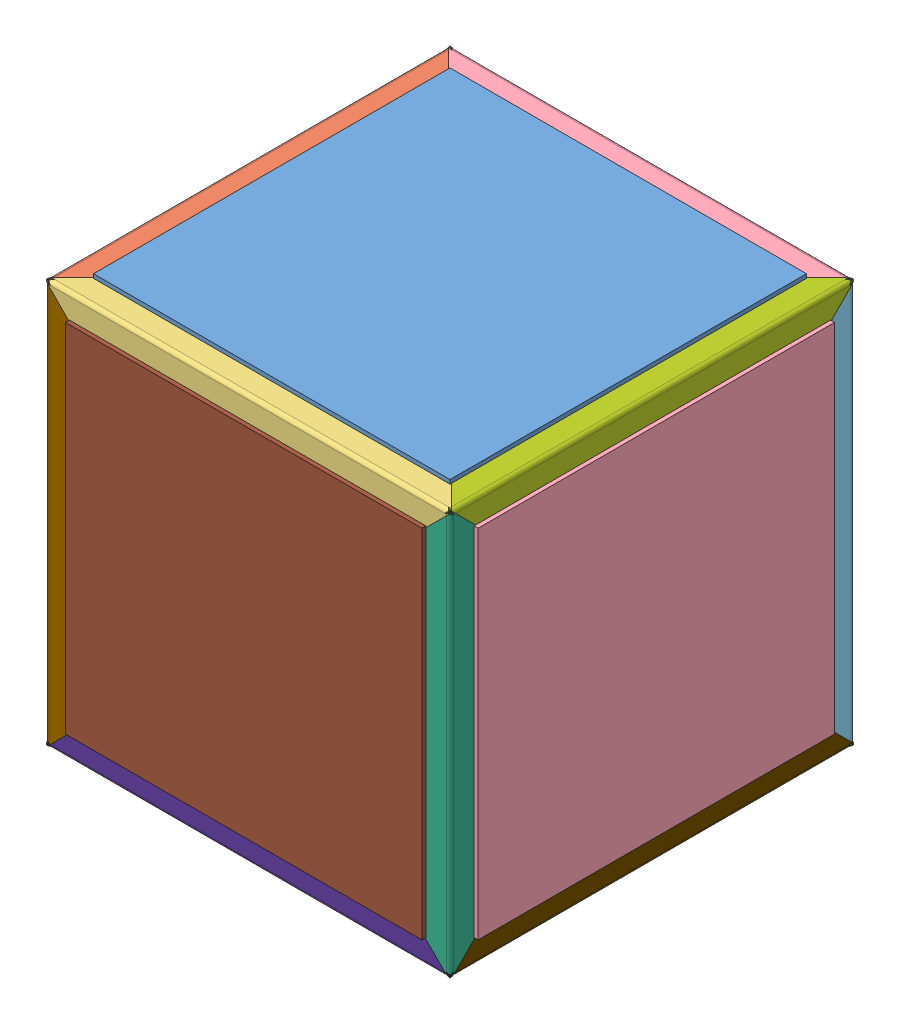
SolidWorks assembly cube_01, configuration cube01. Lengths in mm.
Overall size (163.19 163.19 163.19).
30 component instances, 30 part files, 92 mates.
Components (placement in the parent):
- pr^cube_01-28: pr^cube_01 [cube01] x (-1 0 0) z (0 0 1) size (140.97 1.59 140.97) (virtual)
- dr1^cube_01-55: dr1^cube_01 [cube01] at (-79.4046 80.01 0) x (0 -1 0) z (0 0 1) size (26.01 26.01 160.03) (virtual)
- dr2^cube_01-37: dr2^cube_01 [cube01] at (0 80.01 79.4046) x (0 -1 0) z (1 0 0) size (26.01 26.01 160.03) (virtual)
- dr3^cube_01-33: dr3^cube_01 [cube01] at (0 80.01 -79.4046) x (0 -1 0) z (-1 0 0) size (26.01 26.01 160.03) (virtual)
- br1^cube_01-49: br1^cube_01 [Default] at (0 54.61 -54.61) x (0 0 1) z (-1 0 0) size (50.8 50.8 102.11) (virtual)
- br2^cube_01-61: br2^cube_01 [Default] at (-54.61 54.61 0) size (50.8 50.8 102.11) (virtual)
- br3^cube_01-46: br3^cube_01 [Default] at (0 54.61 54.61) x (0 0 -1) z (1 0 0) size (50.8 50.8 102.11) (virtual)
- pg^cube_01-20: pg^cube_01 [cube01] x (0 -1 0) z (0 0 1) size (140.97 1.59 140.97) (virtual)
- dg1^cube_01-38: dg1^cube_01 [cube01] at (-80.01 0 79.4046) x (1 0 0) z (0 1 0) size (26.01 26.01 160.03) (virtual)
- dg2^cube_01-41: dg2^cube_01 [cube01] at (-80.01 -79.4046 0) size (26.01 26.01 160.03) (virtual)
- dg3^cube_01-34: dg3^cube_01 [cube01] at (-80.01 0 -79.4046) x (1 0 0) z (0 -1 0) size (26.01 26.01 160.03) (virtual)
- bg1^cube_01-47: bg1^cube_01 [Default] at (-54.61 -54.61 0) x (0 1 0) z (0 0 1) size (50.8 50.8 102.11) (virtual)
- bg2^cube_01-44: bg2^cube_01 [Default] at (-54.61 0 54.61) x (0 0 -1) z (0 1 0) size (50.8 50.8 102.11) (virtual)
- bg3^cube_01-40: bg3^cube_01 [Default] at (-54.61 0 -54.61) x (0 0 1) z (0 -1 0) size (50.8 50.8 102.11) (virtual)
- py^cube_01-21: py^cube_01 [cube01] at origin size (140.97 1.59 140.97) (virtual)
- dy1^cube_01-35: dy1^cube_01 [cube01] at (0 -80.01 -79.4046) x (0 1 0) z (1 0 0) size (26.01 26.01 160.03) (virtual)
- dy2^cube_01-39: dy2^cube_01 [cube01] at (0 -80.01 79.4046) x (0 1 0) z (-1 0 0) size (26.01 26.01 160.03) (virtual)
- dy3^cube_01-42: dy3^cube_01 [cube01] at (79.4046 -80.01 0) x (0 1 0) z (0 0 1) size (26.01 26.01 160.03) (virtual)
- by1^cube_01-41: by1^cube_01 [Default] at (0 -54.61 -54.61) x (0 0 1) z (1 0 0) size (50.8 50.8 102.11) (virtual)
- by2^cube_01-45: by2^cube_01 [Default] at (0 -54.61 54.61) x (0 0 -1) z (-1 0 0) size (50.8 50.8 102.11) (virtual)
- by3^cube_01-48: by3^cube_01 [Default] at (54.61 -54.61 0) x (-1 0 0) z (0 0 1) size (50.8 50.8 102.11) (virtual)
- po^cube_01-22: po^cube_01 [cube01] x (0 1 0) z (0 0 1) size (140.97 1.59 140.97) (virtual)
- do1^cube_01-36: do1^cube_01 [cube01] at (80.01 0 -79.4046) x (-1 0 0) z (0 1 0) size (26.01 26.01 160.03) (virtual)
- do2^cube_01-40: do2^cube_01 [cube01] at (80.01 0 79.4046) x (-1 0 0) z (0 -1 0) size (26.01 26.01 160.03) (virtual)
- do3^cube_01-47: do3^cube_01 [cube01] at (80.01 79.4046 0) x (-1 0 0) z (0 0 1) size (26.01 26.01 160.03) (virtual)
- bo1^cube_01-42: bo1^cube_01 [Default] at (54.61 0 -54.61) x (0 0 1) z (0 1 0) size (50.8 50.8 102.11) (virtual)
- bo2^cube_01-46: bo2^cube_01 [Default] at (54.61 0 54.61) x (0 0 -1) z (0 -1 0) size (50.8 50.8 102.11) (virtual)
- bo3^cube_01-62: bo3^cube_01 [Default] at (54.61 54.61 0) x (0 -1 0) z (0 0 1) size (50.8 50.8 102.11) (virtual)
- pc^cube_01-18: pc^cube_01 [cube01] x (-1 0 0) z (0 -1 0) size (140.97 1.59 140.97) (virtual)
- pb^cube_01-21: pb^cube_01 [cube01] x (-1 0 0) z (0 1 0) size (140.97 1.59 140.97) (virtual)
Mates (geometry in assembly coordinates):
- Coincident1: coincident anti-aligned: plane of pr^cube_01-28 through (70.485 80.01 -70.485) normal (0 -1 0); plane of br1^cube_01-49 through (-51.054 80.01 -54.61) normal (0 1 0)
- Coincident2: coincident anti-aligned: plane of pr^cube_01-28 through (70.485 80.01 -70.485) normal (0 -1 0); plane of br2^cube_01-61 through (-54.61 80.01 51.054) normal (0 1 0)
- Coincident3: coincident anti-aligned: plane of pr^cube_01-28 through (70.485 80.01 -70.485) normal (0 -1 0); plane of br3^cube_01-46 through (51.054 80.01 54.61) normal (0 1 0)
- Coincident4: coincident anti-aligned: plane of pr^cube_01-28 through (70.485 80.01 -70.485) normal (0 -1 0); plane of bo3^cube_01-62 through (54.61 80.01 51.054) normal (0 1 0)
- Coincident5: coincident anti-aligned: plane of pr^cube_01-28 through (70.485 80.01 -70.485) normal (0 -1 0); plane of dr3^cube_01-33 through (0 80.01 -159.4146) normal (0 1 0)
- Coincident6: coincident anti-aligned: plane of pr^cube_01-28 through (70.485 80.01 -70.485) normal (0 -1 0); plane of dr1^cube_01-55 through (-159.4146 80.01 0) normal (0 1 0)
- Coincident7: coincident anti-aligned: plane of pr^cube_01-28 through (70.485 80.01 -70.485) normal (0 -1 0); plane of do3^cube_01-47 through (-0.6054 80.01 0) normal (0 1 0)
- Coincident8: coincident anti-aligned: plane of pr^cube_01-28 through (70.485 80.01 -70.485) normal (0 -1 0); plane of dr2^cube_01-37 through (0 80.01 159.4146) normal (0 1 0)
- Coincident34: coincident anti-aligned: plane of pb^cube_01-21 through (70.485 -70.485 -80.01) normal (0 0 1); plane of by1^cube_01-41 through (51.054 -54.61 -80.01) normal (0 0 -1)
- Coincident35: coincident anti-aligned: plane of pb^cube_01-21 through (70.485 -70.485 -80.01) normal (0 0 1); plane of bo1^cube_01-42 through (54.61 51.054 -80.01) normal (0 0 -1)
- Coincident36: coincident anti-aligned: plane of pb^cube_01-21 through (70.485 -70.485 -80.01) normal (0 0 1); plane of br1^cube_01-49 through (-51.054 54.61 -80.01) normal (0 0 -1)
- Coincident37: coincident anti-aligned: plane of pb^cube_01-21 through (70.485 -70.485 -80.01) normal (0 0 1); plane of bg3^cube_01-40 through (-54.61 -51.054 -80.01) normal (0 0 -1)
- Coincident38: coincident anti-aligned: plane of pb^cube_01-21 through (70.485 -70.485 -80.01) normal (0 0 1); plane of dg3^cube_01-34 through (0.6054 0 -80.01) normal (0 0 -1)
- Coincident39: coincident anti-aligned: plane of pb^cube_01-21 through (70.485 -70.485 -80.01) normal (0 0 1); plane of dr3^cube_01-33 through (0 -0.6054 -80.01) normal (0 0 -1)
- Coincident40: coincident anti-aligned: plane of pb^cube_01-21 through (70.485 -70.485 -80.01) normal (0 0 1); plane of do1^cube_01-36 through (-0.6054 0 -80.01) normal (0 0 -1)
- Coincident41: coincident anti-aligned: plane of pb^cube_01-21 through (70.485 -70.485 -80.01) normal (0 0 1); plane of dy1^cube_01-35 through (0 0.6054 -80.01) normal (0 0 -1)
- Coincident42: coincident anti-aligned: plane of pc^cube_01-18 through (70.485 70.485 80.01) normal (0 0 -1); plane of bo2^cube_01-46 through (54.61 -51.054 80.01) normal (0 0 1)
- Coincident43: coincident anti-aligned: plane of pc^cube_01-18 through (70.485 70.485 80.01) normal (0 0 -1); plane of br3^cube_01-46 through (51.054 54.61 80.01) normal (0 0 1)
- Coincident44: coincident anti-aligned: plane of pc^cube_01-18 through (70.485 70.485 80.01) normal (0 0 -1); plane of bg2^cube_01-44 through (-54.61 51.054 80.01) normal (0 0 1)
- Coincident45: coincident anti-aligned: plane of pc^cube_01-18 through (70.485 70.485 80.01) normal (0 0 -1); plane of by2^cube_01-45 through (-51.054 -54.61 80.01) normal (0 0 1)
- Coincident46: coincident anti-aligned: plane of pc^cube_01-18 through (70.485 70.485 80.01) normal (0 0 -1); plane of do2^cube_01-40 through (-0.6054 0 80.01) normal (0 0 1)
- Coincident47: coincident anti-aligned: plane of pc^cube_01-18 through (70.485 70.485 80.01) normal (0 0 -1); plane of dy2^cube_01-39 through (0 0.6054 80.01) normal (0 0 1)
- Coincident48: coincident anti-aligned: plane of pc^cube_01-18 through (70.485 70.485 80.01) normal (0 0 -1); plane of dg1^cube_01-38 through (0.6054 0 80.01) normal (0 0 1)
- Coincident49: coincident anti-aligned: plane of pc^cube_01-18 through (70.485 70.485 80.01) normal (0 0 -1); plane of dr2^cube_01-37 through (0 -0.6054 80.01) normal (0 0 1)
- Coincident50: coincident anti-aligned: plane of pg^cube_01-20 through (-80.01 70.485 -70.485) normal (1 0 0); plane of bg3^cube_01-40 through (-80.01 -51.054 -54.61) normal (-1 0 0)
- Coincident51: coincident anti-aligned: plane of pg^cube_01-20 through (-80.01 70.485 -70.485) normal (1 0 0); plane of bg1^cube_01-47 through (-80.01 -54.61 51.054) normal (-1 0 0)
- Coincident52: coincident anti-aligned: plane of pg^cube_01-20 through (-80.01 70.485 -70.485) normal (1 0 0); plane of bg2^cube_01-44 through (-80.01 51.054 54.61) normal (-1 0 0)
- Coincident53: coincident anti-aligned: plane of pg^cube_01-20 through (-80.01 70.485 -70.485) normal (1 0 0); plane of dr1^cube_01-55 through (-80.01 -0.6054 0) normal (-1 0 0)
- Coincident54: coincident anti-aligned: plane of pg^cube_01-20 through (-80.01 70.485 -70.485) normal (1 0 0); plane of dg3^cube_01-34 through (-80.01 0 -159.4146) normal (-1 0 0)
- Coincident55: coincident anti-aligned: plane of pg^cube_01-20 through (-80.01 70.485 -70.485) normal (1 0 0); plane of dg2^cube_01-41 through (-80.01 -159.4146 0) normal (-1 0 0)
- Coincident56: coincident anti-aligned: plane of pg^cube_01-20 through (-80.01 70.485 -70.485) normal (1 0 0); plane of dg1^cube_01-38 through (-80.01 0 159.4146) normal (-1 0 0)
- Coincident99: coincident anti-aligned: plane of pg^cube_01-20 through (-80.01 70.485 -70.485) normal (1 0 0); plane of br2^cube_01-61 through (-80.01 54.61 51.054) normal (-1 0 0)
- Coincident57: coincident anti-aligned: plane of py^cube_01-21 through (-70.485 -80.01 -70.485) normal (0 1 0); plane of by3^cube_01-48 through (54.61 -80.01 51.054) normal (0 -1 0)
- Coincident58: coincident anti-aligned: plane of py^cube_01-21 through (-70.485 -80.01 -70.485) normal (0 1 0); plane of by2^cube_01-45 through (-51.054 -80.01 54.61) normal (0 -1 0)
- Coincident59: coincident anti-aligned: plane of py^cube_01-21 through (-70.485 -80.01 -70.485) normal (0 1 0); plane of bg1^cube_01-47 through (-54.61 -80.01 51.054) normal (0 -1 0)
- Coincident60: coincident anti-aligned: plane of py^cube_01-21 through (-70.485 -80.01 -70.485) normal (0 1 0); plane of by1^cube_01-41 through (51.054 -80.01 -54.61) normal (0 -1 0)
- Coincident61: coincident anti-aligned: plane of py^cube_01-21 through (-70.485 -80.01 -70.485) normal (0 1 0); plane of dy3^cube_01-42 through (159.4146 -80.01 0) normal (0 -1 0)
- Coincident62: coincident anti-aligned: plane of py^cube_01-21 through (-70.485 -80.01 -70.485) normal (0 1 0); plane of dy2^cube_01-39 through (0 -80.01 159.4146) normal (0 -1 0)
- Coincident63: coincident anti-aligned: plane of py^cube_01-21 through (-70.485 -80.01 -70.485) normal (0 1 0); plane of dg2^cube_01-41 through (0.6054 -80.01 0) normal (0 -1 0)
- Coincident64: coincident anti-aligned: plane of py^cube_01-21 through (-70.485 -80.01 -70.485) normal (0 1 0); plane of dy1^cube_01-35 through (0 -80.01 -159.4146) normal (0 -1 0)
- Coincident65: coincident anti-aligned: plane of po^cube_01-22 through (80.01 -70.485 -70.485) normal (-1 0 0); plane of bo1^cube_01-42 through (80.01 51.054 -54.61) normal (1 0 0)
- Coincident66: coincident anti-aligned: plane of po^cube_01-22 through (80.01 -70.485 -70.485) normal (-1 0 0); plane of by3^cube_01-48 through (80.01 -54.61 51.054) normal (1 0 0)
- Coincident67: coincident anti-aligned: plane of po^cube_01-22 through (80.01 -70.485 -70.485) normal (-1 0 0); plane of bo2^cube_01-46 through (80.01 -51.054 54.61) normal (1 0 0)
- Coincident68: coincident anti-aligned: plane of po^cube_01-22 through (80.01 -70.485 -70.485) normal (-1 0 0); plane of bo3^cube_01-62 through (80.01 54.61 51.054) normal (1 0 0)
- Coincident69: coincident anti-aligned: plane of po^cube_01-22 through (80.01 -70.485 -70.485) normal (-1 0 0); plane of do2^cube_01-40 through (80.01 0 159.4146) normal (1 0 0)
- Coincident70: coincident anti-aligned: plane of po^cube_01-22 through (80.01 -70.485 -70.485) normal (-1 0 0); plane of do3^cube_01-47 through (80.01 159.4146 0) normal (1 0 0)
- Coincident71: coincident anti-aligned: plane of po^cube_01-22 through (80.01 -70.485 -70.485) normal (-1 0 0); plane of do1^cube_01-36 through (80.01 0 -159.4146) normal (1 0 0)
- Coincident72: coincident anti-aligned: plane of po^cube_01-22 through (80.01 -70.485 -70.485) normal (-1 0 0); plane of dy3^cube_01-42 through (80.01 0.6054 0) normal (1 0 0)
- Coincident73: coincident aligned: plane of assembly through (0 0 0) normal (0 0 1); plane of dy3^cube_01-42 through (79.4046 -80.01 0) normal (0 0 1)
- Coincident74: coincident aligned: plane of assembly through (0 0 0) normal (0 0 1); plane of by3^cube_01-48 through (54.61 -54.61 0) normal (0 0 1)
- Coincident75: coincident aligned: plane of assembly through (0 0 0) normal (0 0 1); plane of bo3^cube_01-62 through (54.61 54.61 0) normal (0 0 1)
- Coincident76: coincident aligned: plane of assembly through (0 0 0) normal (0 0 1); plane of do3^cube_01-47 through (80.01 79.4046 0) normal (0 0 1)
- Coincident77: coincident aligned: plane of assembly through (0 0 0) normal (0 0 1); plane of dg2^cube_01-41 through (-80.01 -79.4046 0) normal (0 0 1)
- Coincident78: coincident aligned: plane of assembly through (0 0 0) normal (0 0 1); plane of bg1^cube_01-47 through (-54.61 -54.61 0) normal (0 0 1)
- Coincident79: coincident aligned: plane of assembly through (0 0 0) normal (0 0 1); plane of dr1^cube_01-55 through (-79.4046 80.01 0) normal (0 0 1)
- Coincident80: coincident aligned: plane of assembly through (0 0 0) normal (0 0 1); plane of br2^cube_01-61 through (-54.61 54.61 0) normal (0 0 1)
- Coincident81: coincident aligned: plane of assembly through (0 0 0) normal (0 1 0); plane of bo1^cube_01-42 through (54.61 0 -54.61) normal (0 1 0)
- Coincident82: coincident aligned: plane of assembly through (0 0 0) normal (0 1 0); plane of py^cube_01-21 through (0 0 0) normal (0 1 0)
- Coincident83: coincident aligned: plane of assembly through (0 0 0) normal (0 1 0); plane of do1^cube_01-36 through (80.01 0 -79.4046) normal (0 1 0)
- Coincident84: coincident anti-aligned: plane of assembly through (0 0 0) normal (0 1 0); plane of bg3^cube_01-40 through (-54.61 0 -54.61) normal (0 -1 0)
- Coincident85: coincident anti-aligned: plane of assembly through (0 0 0) normal (0 1 0); plane of dg3^cube_01-34 through (-80.01 0 -79.4046) normal (0 -1 0)
- Coincident86: coincident aligned: plane of assembly through (0 0 0) normal (0 1 0); plane of dg1^cube_01-38 through (-80.01 0 79.4046) normal (0 1 0)
- Coincident87: coincident aligned: plane of assembly through (0 0 0) normal (0 1 0); plane of bg2^cube_01-44 through (-54.61 0 54.61) normal (0 1 0)
- Coincident88: coincident anti-aligned: plane of assembly through (0 0 0) normal (0 1 0); plane of bo2^cube_01-46 through (54.61 0 54.61) normal (0 -1 0)
- Coincident89: coincident anti-aligned: plane of assembly through (0 0 0) normal (0 1 0); plane of do2^cube_01-40 through (80.01 0 79.4046) normal (0 -1 0)
- Coincident90: coincident anti-aligned: plane of assembly through (0 0 0) normal (1 0 0); plane of by2^cube_01-45 through (0 -54.61 54.61) normal (-1 0 0)
- Coincident91: coincident anti-aligned: plane of assembly through (0 0 0) normal (1 0 0); plane of dy2^cube_01-39 through (0 -80.01 79.4046) normal (-1 0 0)
- Coincident92: coincident aligned: plane of assembly through (0 0 0) normal (1 0 0); plane of pg^cube_01-20
- Coincident93: coincident aligned: plane of assembly through (0 0 0) normal (1 0 0); plane of dr2^cube_01-37 through (0 80.01 79.4046) normal (1 0 0)
- Coincident94: coincident aligned: plane of assembly through (0 0 0) normal (1 0 0); plane of br3^cube_01-46 through (0 54.61 54.61) normal (1 0 0)
- Coincident95: coincident anti-aligned: plane of assembly through (0 0 0) normal (1 0 0); plane of dr3^cube_01-33 through (0 80.01 -79.4046) normal (-1 0 0)
- Coincident96: coincident anti-aligned: plane of assembly through (0 0 0) normal (1 0 0); plane of br1^cube_01-49 through (0 54.61 -54.61) normal (-1 0 0)
- Coincident97: coincident aligned: plane of assembly through (0 0 0) normal (1 0 0); plane of by1^cube_01-41 through (0 -54.61 -54.61) normal (1 0 0)
- Coincident98: coincident aligned: plane of assembly through (0 0 0) normal (1 0 0); plane of dy1^cube_01-35 through (0 -80.01 -79.4046) normal (1 0 0)
- Coincident100: coincident anti-aligned: plane of pr^cube_01-28; plane of assembly through (0 0 0) normal (1 0 0)
- Coincident101: coincident aligned: plane of pr^cube_01-28 through (0 0 0) normal (0 0 1); plane of assembly through (0 0 0) normal (0 0 1)
- Coincident102: coincident anti-aligned: plane of pr^cube_01-28; plane of assembly through (0 0 0) normal (0 1 0)
- Coincident106: coincident anti-aligned: plane of pg^cube_01-20; plane of assembly through (0 0 0) normal (0 1 0)
- Coincident107: coincident aligned: plane of pg^cube_01-20; plane of assembly through (0 0 0) normal (1 0 0)
- Coincident108: coincident aligned: plane of pg^cube_01-20 through (0 0 0) normal (0 0 1); plane of assembly through (0 0 0) normal (0 0 1)
- Coincident109: coincident aligned: plane of py^cube_01-21 through (0 0 0) normal (0 0 1); plane of assembly through (0 0 0) normal (0 0 1)
- Coincident110: coincident aligned: plane of py^cube_01-21 through (0 0 0) normal (0 1 0); plane of assembly through (0 0 0) normal (0 1 0)
- Coincident111: coincident aligned: plane of py^cube_01-21 through (0 0 0) normal (1 0 0); plane of assembly through (0 0 0) normal (1 0 0)
- Coincident112: coincident aligned: plane of po^cube_01-22 through (0 0 0) normal (0 0 1); plane of assembly through (0 0 0) normal (0 0 1)
- Coincident113: coincident anti-aligned: plane of po^cube_01-22; plane of assembly through (0 0 0) normal (1 0 0)
- Coincident114: coincident aligned: plane of po^cube_01-22; plane of assembly through (0 0 0) normal (0 1 0)
- Coincident115: coincident anti-aligned: plane of pc^cube_01-18 through (0 0 0) normal (0 -1 0); plane of assembly through (0 0 0) normal (0 1 0)
- Coincident116: coincident anti-aligned: plane of pc^cube_01-18; plane of assembly through (0 0 0) normal (0 0 1)
- Coincident117: coincident anti-aligned: plane of pc^cube_01-18; plane of assembly through (0 0 0) normal (1 0 0)
- Coincident118: coincident aligned: plane of pb^cube_01-21 through (0 0 0) normal (0 1 0); plane of assembly through (0 0 0) normal (0 1 0)
- Coincident119: coincident aligned: plane of pb^cube_01-21; plane of assembly through (0 0 0) normal (0 0 1)
- Coincident120: coincident anti-aligned: line of pb^cube_01-21 through (0.8731 -0.8731 0) axis (0 0 -1); plane of assembly through (0 0 0) normal (1 0 0)
